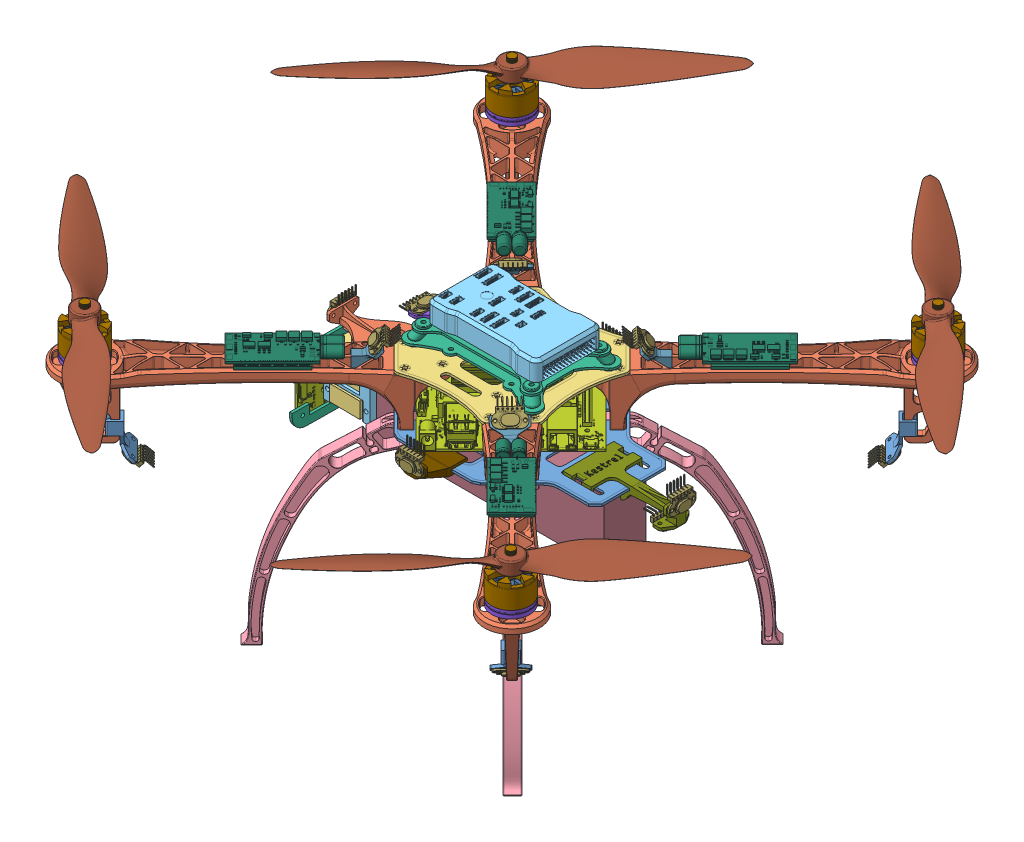
SolidWorks assembly KestrelAssem, configuration Default. Lengths in mm.
Overall size (525.79 228.99 525.79).
72 component instances, 26 part files, 118 mates.
Components (placement in the parent):
- Base bottom-1: Base bottom [Default] at (67.5563 86.9564 146.6689) size (182 1.6 118)
- arm-1: arm [Default] at (165.9237 126.3564 245.0469) x (-0.707107 0 0.707107) z (-0.707107 0 -0.707107) size (40.75 55.34 213.92)
- arm-2: arm [Default] at (-30.8217 126.3564 245.0362) x (-0.707107 0 -0.707107) z (0.707107 0 -0.707107) size (40.75 55.34 213.92)
- arm-3: arm [Default] at (165.9344 126.3564 48.3015) x (0.707107 0 0.707107) z (-0.707107 0 0.707107) size (40.75 55.34 213.92)
- arm-4: arm [Default] at (-30.811 126.3564 48.2908) x (0.707107 0 -0.707107) z (0.707107 0 0.707107) size (40.75 55.34 213.92)
- Base Top-1: Base Top [Default] at (67.5563 125.3865 146.6689) x (0 0 -1) z (1 0 0) size (108.15 1.65 108.15)
- patadrone3definitiva-1: patadrone3definitiva [Predeterminado] at (172.5269 -57.1369 48.4158) x (-0.707107 0 0.707107) z (-0.707107 0 -0.707107) size (111.61 160.57 31.98)
- patadrone3definitiva-2: patadrone3definitiva [Predeterminado] at (-30.3432 -57.1369 41.3447) x (0.707107 0 0.707107) z (-0.707107 0 0.707107) size (111.61 160.57 31.98)
- patadrone3definitiva-3: patadrone3definitiva [Predeterminado] at (165.8094 -57.1369 251.6394) x (-0.707107 0 -0.707107) z (0.707107 0 -0.707107) size (111.61 160.57 31.98)
- patadrone3definitiva-4: patadrone3definitiva [Predeterminado] at (-37.4142 -57.1369 244.9219) x (0.707107 0 -0.707107) z (0.707107 0 0.707107) size (111.61 160.57 31.98)
- pixhawk-1: pixhawk [Default] at (69.0326 138.9713 146.4116) x (0 0 1) z (-1 0 0) size (49.7 16 82)
- base_pixhawk-1: base_pixhawk [Predeterminado] at (67.5563 126.89 137.1312) x (0 0 -1) z (1 0 0) size (70 13.5 101)
- Jetson nano_fixed-2: Jetson nano_fixed [Default] at (50.0251 91.2381 194.8479) x (0.707107 0 -0.707107) z (0 1 0) size (100 81.03 30.51)
- emax2213-3: emax2213 [Default] at (-115.5179 114.2807 302.8982) x (0.53753 0 -0.843245) z (0.843245 0 0.53753) size (30.02 35.87 30.02)
  - Part27-1: Part27 [Default] at (10.7352 10.5257 21.811) size (27.95 6.6 27.95)
  - rotor-1: rotor [Default] at (10.7352 16.1257 21.811) x (-0.046958 0 -0.998897) z (0.998897 0 -0.046958) size (28.06 30.27 28.06)
  - stator-1: stator [Default] at (10.7352 14.6357 21.811) x (-0.821098 0 -0.570787) z (0.570787 0 -0.821098) size (21.57 13.8 21.57)
- Propeller 10x45-3: Propeller 10x45 [Default] at (-91.3554 152.6764 305.5699) x (0.684738 0 -0.72879) z (0.72879 0 0.684738) size (33.64 14.19 254.22)
- TOF400C-2: TOF400C [Défaut] at (16.6624 134.5984 197.0939) x (-0.726351 -0.001282 -0.687323) z (-0.486669 0.707107 0.512985) size (20 18.23 7.52)
- Battery-1: Battery [Default] at (67.5563 62.1564 131.356) x (1 0 0) z (0 -1 0) size (169 31.5 48)
- Top Sensor Mount-1: Top Sensor Mount [Default] at (14.5099 121.5155 199.3264) x (-0.688254 0 0.72547) z (-0.72547 0 -0.688254) size (17.07 22.27 22)
- ESC 26X50mm-1: ESC 26X50mm [Default] at (-21.2525 131.4243 235.9148) x (-0.707107 0 0.707107) z (0 1 0) size (62.87 25.9 10.08)
- Rear Horizontal Sensor Mount-1: Rear Horizontal Sensor Mount [Default] at (145.7563 87.8564 147.106) x (0 0 -1) z (1 0 0) size (39.5 19.31 69)
- TOF400C-8: TOF400C [Défaut] at (194.3563 93.7637 147.081) x (0 0 1) z (1 0 0) size (20 18.23 7.52)
- TOF400C-9: TOF400C [Défaut] at (67.5813 93.6637 68.2503) x (1 0 0) z (0 0 -1) size (20 18.23 7.52)
- Side Horizontal Mount-1: Side Horizontal Mount [Default] at (67.5563 87.7564 89.8503) x (-1 0 0) z (0 0 -1) size (26 12.61 27.76)
- Side Horizontal Mount Pt2-1: Side Horizontal Mount Pt2 [Default] at (67.5563 87.7564 199.3503) size (34.53 12.61 31.5)
- TOF400C-14: TOF400C [Défaut] at (67.5813 93.6637 222.9503) x (-1 0 0) z (0 0 1) size (20 18.23 7.52)
- Angle Down Mount-1: Angle Down Mount [Default] at (-82.2131 82.3894 291.9609) x (-0.707107 0 -0.707107) z (0.707107 0 -0.707107) size (22 23.82 16.77)
- TOF400C-15: TOF400C [Défaut] at (-74.539 64.8571 288.8477) x (0.707107 0 0.707107) z (-0.498006 -0.709916 0.498006) size (20 18.23 7.52)
- Forward Horizontal Sensor Mount-1: Forward Horizontal Sensor Mount [Default] at (-10.6437 87.8564 147.106) x (0 0 1) z (-1 0 0) size (40.84 19.31 71.66)
- TOF400C-19: TOF400C [Défaut] at (-59.2437 93.7637 147.081) x (0 0 -1) z (-1 0 0) size (20 18.23 7.52)
- SG90-servo-1: SG90-servo [Varsayılan] at (-47.0683 69.2064 147.0402) x (0.999938 0 0.011104) z (0 -1 0) size (33 11.95 30.5)
- Servo Arm-1: Servo Arm [Peça] at (-41.1437 84.1564 147.106) size (34.5 3.8 16.7)
- Camera Mount pt2-1: Camera Mount pt2 [Default] at (-61.5674 69.2064 146.8792) x (-0.999938 0 -0.011104) z (0.011104 0 -0.999938) size (35 33.25 15.8)
- SG90-servo-2: SG90-servo [Varsayılan] at (-46.9806 43.8564 139.1406) x (-0.999938 0 -0.011104) z (-0.011104 0 0.999938) size (33 11.95 30.5)
- Servo Arm-2: Servo Arm [Peça] at (-52.7392 43.8564 124.1258) x (-0.999816 -0.015644 -0.011102) z (0.015643 -0.999878 0.000174) size (34.5 3.8 16.7)
- Camera Mount Pt3-1: Camera Mount Pt3 [Default] at (-52.7392 43.8564 124.1258) x (0.011104 0 -0.999938) z (0.999816 0.015644 0.011102) size (49.7 49.7 38.4)
- Camera-1: Camera [Default] at (-74.4135 38.4187 136.2155) x (-0.015643 0.999878 -0.000174) z (-0.999816 -0.015644 -0.011102) size (38 38 23.66)
- Upward Sensor Mount-1: Upward Sensor Mount [Default] at (32.5563 126.2115 146.6689) x (0 0 1) z (-1 0 0) size (22 5.7 33.62)
- TOF400C-20: TOF400C [Défaut] at (3.699 126.9615 146.6439) x (0 0 1) z (0 1 0) size (20 18.23 7.52)
- TOF400C-21: TOF400C [Défaut] at (185.999 78.5564 147.081) x (0 0 -1) z (0 -1 0) size (20 18.23 7.52)
- TOF400C-5: TOF400C [Défaut] at (117.5443 134.5984 197.9999) x (-0.687323 -0.001282 0.726351) z (0.512985 0.707107 0.486669) size (20 18.23 7.52)
- TOF400C-6: TOF400C [Défaut] at (118.4503 134.5984 97.118) x (0.726351 -0.001282 0.687323) z (0.486669 0.707107 -0.512985) size (20 18.23 7.52)
- TOF400C-7: TOF400C [Défaut] at (17.5684 134.5984 96.212) x (0.687323 -0.001282 -0.726351) z (-0.512985 0.707107 -0.486669) size (20 18.23 7.52)
- Top Sensor Mount-2: Top Sensor Mount [Default] at (119.7768 121.5155 200.1524) x (0.72547 0 0.688254) z (-0.688254 0 0.72547) size (17.07 22.27 22)
- Top Sensor Mount-3: Top Sensor Mount [Default] at (120.6028 121.5155 94.8855) x (0.688254 0 -0.72547) z (0.72547 0 0.688254) size (17.07 22.27 22)
- Top Sensor Mount-4: Top Sensor Mount [Default] at (15.3359 121.5155 94.0595) x (-0.72547 0 -0.688254) z (0.688254 0 -0.72547) size (17.07 22.27 22)
- emax2213-5: emax2213 [Default] at (223.3486 114.2807 330.1802) x (-0.843245 0 -0.53753) z (0.53753 0 -0.843245) size (30.02 35.87 30.02)
  - Part27-1: Part27 [Default] at (10.7352 10.5257 21.811) size (27.95 6.6 27.95)
  - rotor-1: rotor [Default] at (10.7352 16.1257 21.811) x (-0.046958 0 -0.998897) z (0.998897 0 -0.046958) size (28.06 30.27 28.06)
  - stator-1: stator [Default] at (10.7352 14.6357 21.811) x (-0.821098 0 -0.570787) z (0.570787 0 -0.821098) size (21.57 13.8 21.57)
- emax2213-6: emax2213 [Default] at (250.6306 114.2807 -8.6863) x (-0.53753 0 0.843245) z (-0.843245 0 -0.53753) size (30.02 35.87 30.02)
  - Part27-1: Part27 [Default] at (10.7352 10.5257 21.811) size (27.95 6.6 27.95)
  - rotor-1: rotor [Default] at (10.7352 16.1257 21.811) x (-0.046958 0 -0.998897) z (0.998897 0 -0.046958) size (28.06 30.27 28.06)
  - stator-1: stator [Default] at (10.7352 14.6357 21.811) x (-0.821098 0 -0.570787) z (0.570787 0 -0.821098) size (21.57 13.8 21.57)
- emax2213-7: emax2213 [Default] at (-88.2359 114.2807 -35.9683) x (0.843245 0 0.53753) z (-0.53753 0 0.843245) size (30.02 35.87 30.02)
  - Part27-1: Part27 [Default] at (10.7352 10.5257 21.811) size (27.95 6.6 27.95)
  - rotor-1: rotor [Default] at (10.7352 16.1257 21.811) x (-0.046958 0 -0.998897) z (0.998897 0 -0.046958) size (28.06 30.27 28.06)
  - stator-1: stator [Default] at (10.7352 14.6357 21.811) x (-0.821098 0 -0.570787) z (0.570787 0 -0.821098) size (21.57 13.8 21.57)
- Propeller 10x45-5: Propeller 10x45 [Default] at (226.0203 152.6764 306.0177) x (-0.72879 0 -0.684738) z (0.684738 0 -0.72879) size (33.64 14.19 254.22)
- Propeller 10x45-6: Propeller 10x45 [Default] at (226.4681 152.6764 -11.358) x (-0.684738 0 0.72879) z (-0.72879 0 -0.684738) size (33.64 14.19 254.22)
- Propeller 10x45-7: Propeller 10x45 [Default] at (-90.9076 152.6764 -11.8058) x (0.72879 0 0.684738) z (-0.684738 0 0.72879) size (33.64 14.19 254.22)
- ESC 26X50mm-2: ESC 26X50mm [Default] at (156.3652 131.4243 235.9148) x (0.707107 0 0.707107) z (0 1 0) size (62.87 25.9 10.08)
- ESC 26X50mm-3: ESC 26X50mm [Default] at (156.3652 131.4243 58.2971) x (0.707107 0 -0.707107) z (0 1 0) size (62.87 25.9 10.08)
- ESC 26X50mm-4: ESC 26X50mm [Default] at (-21.2525 131.4243 58.2971) x (-0.707107 0 -0.707107) z (0 1 0) size (62.87 25.9 10.08)
- TOF400C-16: TOF400C [Défaut] at (-74.1854 64.8571 5.0106) x (-0.707107 0 0.707107) z (-0.498006 -0.709916 -0.498006) size (20 18.23 7.52)
- TOF400C-17: TOF400C [Défaut] at (209.6517 64.8571 5.3642) x (-0.707107 0 -0.707107) z (0.498006 -0.709916 -0.498006) size (20 18.23 7.52)
- TOF400C-18: TOF400C [Défaut] at (209.298 64.8571 289.2013) x (0.707107 0 -0.707107) z (0.498006 -0.709916 0.498006) size (20 18.23 7.52)
- Angle Down Mount-2: Angle Down Mount [Default] at (-77.2986 82.3894 -2.6635) x (0.707107 0 -0.707107) z (0.707107 0 0.707107) size (22 23.82 16.77)
- Angle Down Mount-3: Angle Down Mount [Default] at (217.3258 82.3894 2.251) x (0.707107 0 0.707107) z (-0.707107 0 0.707107) size (22 23.82 16.77)
- Angle Down Mount-4: Angle Down Mount [Default] at (212.4113 82.3894 296.8754) x (-0.707107 0 0.707107) z (-0.707107 0 -0.707107) size (22 23.82 16.77)
Mates (geometry in assembly coordinates):
- Coincident2: coincident anti-aligned: plane of Base bottom-1 through (4.0563 87.7564 186.9169) normal (0 1 0); plane of arm-1 through (104.3913 87.7564 193.9796) normal (0 -1 0)
- Coincident3: coincident anti-aligned: axis of Base bottom-1 through (99.5883 86.1554 193.1965) axis (0 1 0); line of arm-1 through (99.5883 92.7564 193.1965) axis (0 -1 0)
- Coincident4: coincident anti-aligned: line of Base bottom-1 through (114.084 86.1554 178.7008) axis (0 1 0); line of arm-1 through (114.084 92.7564 178.7008) axis (0 -1 0)
- Coincident5: coincident anti-aligned: plane of Base bottom-1 through (4.0563 87.7564 186.9169) normal (0 1 0); plane of arm-2 through (35.6249 87.7564 197.7501) normal (0 -1 0)
- Coincident6: coincident anti-aligned: line of Base bottom-1 through (21.0287 86.1554 178.7008) axis (0 1 0); line of arm-2 through (21.0287 92.7564 178.7008) axis (0 -1 0)
- Coincident7: coincident anti-aligned: line of Base bottom-1 through (35.5244 86.1554 193.1965) axis (0 1 0); line of arm-2 through (35.5244 92.7564 193.1965) axis (0 -1 0)
- Coincident8: coincident anti-aligned: line of Base bottom-1 through (114.084 86.1554 114.6369) axis (0 1 0); line of arm-3 through (114.084 92.7564 114.6369) axis (0 -1 0)
- Coincident9: coincident anti-aligned: plane of Base bottom-1 through (4.0563 87.7564 186.9169) normal (0 1 0); plane of arm-3 through (114.8671 87.7564 109.8339) normal (0 -1 0)
- Coincident10: coincident anti-aligned: line of Base bottom-1 through (99.5883 86.1554 100.1412) axis (0 1 0); line of arm-3 through (99.5883 92.7564 100.1412) axis (0 -1 0)
- Coincident13: coincident anti-aligned: line of Base bottom-1 through (35.5244 86.1554 100.1412) axis (0 1 0); line of arm-4 through (35.5244 92.7564 100.1412) axis (0 -1 0)
- Coincident14: coincident anti-aligned: plane of Base bottom-1 through (4.0563 87.7564 186.9169) normal (0 1 0); plane of arm-4 through (30.7214 87.7564 99.3581) normal (0 -1 0)
- Coincident15: coincident anti-aligned: line of Base bottom-1 through (21.0287 86.1554 114.6369) axis (0 1 0); line of arm-4 through (21.0287 92.7564 114.6369) axis (0 -1 0)
- Coincident16: coincident anti-aligned: plane of arm-1 through (121.2204 124.5615 177.999) normal (0 1 0); plane of Base Top-1 through (18.1568 124.5615 114.9285) normal (0 -1 0)
- Coincident17: coincident aligned: line of arm-1 through (99.0226 119.5615 194.7521) axis (0 1 0); line of Base Top-1 through (99.0226 124.5605 194.7521) axis (0 1 0)
- Coincident18: coincident aligned: line of arm-1 through (115.6396 119.5615 178.1351) axis (0 1 0); line of Base Top-1 through (115.6396 124.5605 178.1351) axis (0 1 0)
- Concentric1: concentric aligned: circle of Base bottom-1; circle of patadrone3definitiva-1
- Coincident19: coincident anti-aligned: plane of Base bottom-1 through (4.0563 86.1564 186.9169) normal (0 -1 0); plane of patadrone3definitiva-1 through (109.2957 86.1564 97.5049) normal (0 1 0)
- Parallel1: parallel aligned: line of Base bottom-1 through (123.9835 86.1564 115.344) axis (-0.707107 0 -0.707107); line of patadrone3definitiva-1 through (106.6908 86.1564 98.8433) axis (-0.707107 0 -0.707107)
- Concentric3: concentric aligned: circle of Base bottom-1; circle of patadrone3definitiva-2
- Coincident20: coincident anti-aligned: plane of Base bottom-1 through (4.0563 86.1564 186.9169) normal (0 -1 0); plane of patadrone3definitiva-2 through (18.7459 86.1564 104.576) normal (0 1 0)
- Parallel2: parallel aligned: line of Base bottom-1 through (30.9282 86.1564 95.545) axis (-0.707107 0 0.707107); line of patadrone3definitiva-2 through (32.7384 86.1564 94.5268) axis (-0.707107 0 0.707107)
- Concentric5: concentric aligned: circle of Base bottom-1; circle of patadrone3definitiva-4
- Coincident22: coincident anti-aligned: plane of Base bottom-1 through (4.0563 86.1564 186.9169) normal (0 -1 0); plane of patadrone3definitiva-4 through (25.817 86.1564 195.8328) normal (0 1 0)
- Parallel5: parallel aligned: line of Base bottom-1 through (12.0544 86.1564 178.9189) axis (0.707107 0 0.707107); line of patadrone3definitiva-4 through (28.4219 86.1564 194.4944) axis (0.707107 0 0.707107)
- Concentric6: concentric aligned: circle of Base bottom-1; circle of patadrone3definitiva-3
- Coincident23: coincident anti-aligned: plane of Base bottom-1 through (4.0563 86.1564 186.9169) normal (0 -1 0); plane of patadrone3definitiva-3 through (116.7203 86.1564 188.4082) normal (0 1 0)
- Parallel6: parallel aligned: line of Base bottom-1 through (99.8063 86.1564 202.1708) axis (0.707107 0 -0.707107); line of patadrone3definitiva-3 through (102.7278 86.1564 198.4574) axis (0.707107 0 -0.707107)
- Concentric7: concentric anti-aligned: circle of arm-3; circle of emax2213-1/Part27-1
- Coincident24: coincident anti-aligned: plane of arm-3 through (207.1853 124.8064 -19.441) normal (0 1 0); plane of emax2213-1/Part27-1 through (226.4681 124.8064 -12.2322) normal (0 -1 0)
- Concentric8: concentric anti-aligned: circle of arm-1; circle of emax2213-2/Part27-1
- Coincident25: coincident anti-aligned: plane of arm-1 through (233.6662 124.8064 286.2978) normal (0 1 0); plane of emax2213-2/Part27-1 through (226.4574 124.8064 305.5806) normal (0 -1 0)
- Concentric9: concentric anti-aligned: circle of arm-2; circle of emax2213-3/Part27-1
- Coincident26: coincident anti-aligned: plane of arm-2 through (-72.0726 124.8064 312.7787) normal (0 1 0); plane of emax2213-3/Part27-1 through (-91.3554 124.8064 305.5699) normal (0 -1 0)
- Concentric10: concentric anti-aligned: circle of arm-4; circle of emax2213-4/Part27-1
- Coincident27: coincident anti-aligned: plane of arm-4 through (-98.5535 124.8064 7.0399) normal (0 1 0); plane of emax2213-4/Part27-1 through (-91.3447 124.8064 -12.2429) normal (0 -1 0)
- Concentric11: concentric aligned: circle of emax2213-4/rotor-1; circle of Propeller 10x45-4
- Coincident28: coincident anti-aligned: plane of emax2213-4/rotor-1 through (-91.3447 147.6764 -12.2429) normal (0 1 0); plane of Propeller 10x45-4 through (-91.3447 147.6764 -12.2429) normal (0 -1 0)
- Concentric12: concentric aligned: circle of emax2213-3/rotor-1; circle of Propeller 10x45-3
- Coincident29: coincident anti-aligned: plane of emax2213-3/rotor-1 through (-91.3554 147.6764 305.5699) normal (0 1 0); plane of Propeller 10x45-3 through (-91.3554 147.6764 305.5699) normal (0 -1 0)
- Concentric13: concentric aligned: circle of emax2213-2/rotor-1; circle of Propeller 10x45-2
- Coincident30: coincident anti-aligned: plane of emax2213-2/rotor-1 through (226.4574 147.6764 305.5806) normal (0 1 0); plane of Propeller 10x45-2 through (226.4574 147.6764 305.5806) normal (0 -1 0)
- Concentric14: concentric aligned: circle of emax2213-1/rotor-1; circle of Propeller 10x45-1
- Coincident31: coincident anti-aligned: plane of emax2213-1/rotor-1 through (226.4681 147.6764 -12.2322) normal (0 1 0); plane of Propeller 10x45-1 through (226.4681 147.6764 -12.2322) normal (0 -1 0)
- Parallel8: parallel aligned: plane of Top Sensor Mount-1 through (14.5099 121.5155 199.3264) normal (0 1 0)
- Concentric15: concentric aligned: circle of TOF400C-2; circle of Top Sensor Mount-1
- Coincident37: coincident anti-aligned: plane of TOF400C-2 through (20.9493 134.1812 200.5664) normal (0.486669 -0.707107 -0.512985); plane of Top Sensor Mount-1 through (6.4052 136.3057 183.8399) normal (-0.486669 0.707107 0.512985)
- Coincident40: coincident: point of arm-2; line of ESC 26X50mm-1 through (-44.3113 125.4243 242.1277) axis (0.707107 0 0.707107)
- Coincident41: coincident: point of arm-2; line of ESC 26X50mm-1 through (-44.3113 125.4243 242.1277) axis (0.707107 0 0.707107)
- Parallel9: parallel anti-aligned: plane of ESC 26X50mm-1 through (-21.2243 125.4243 236.0113) normal (0 -1 0)
- Coincident42: coincident: line of ESC 26X50mm-1 through (-38.9301 131.4243 253.5924) axis (0.707107 0 -0.707107)
- Coincident43: coincident anti-aligned: plane of Base bottom-1 through (4.0563 86.1564 186.9169) normal (0 -1 0); plane of Battery-1 through (-16.9437 86.1564 162.856) normal (0 1 0)
- Coincident44: coincident anti-aligned: plane of Battery-1 through (67.5563 62.1564 131.356) normal (1 0 0)
- Distance1: distance = 15.75 mm aligned: plane of Battery-1 through (67.5563 62.1564 131.356) normal (0 0 1)
- Coincident46: coincident aligned: line of Base bottom-1 through (124.7563 86.1564 166.106) axis (1 0 0); line of Rear Horizontal Sensor Mount-1 through (138.7563 86.1564 166.106) axis (1 0 0)
- Coincident47: coincident anti-aligned: line of Base bottom-1 through (150.5563 86.1564 128.106) axis (-1 0 0); line of Rear Horizontal Sensor Mount-1 through (138.7563 86.1564 128.106) axis (1 0 0)
- Coincident48: coincident anti-aligned: plane of Battery-1 through (152.0563 86.1564 162.856) normal (1 0 0); plane of Rear Horizontal Sensor Mount-1 through (152.0563 84.1564 150.606) normal (-1 0 0)
- Concentric17: concentric aligned: circle of Rear Horizontal Sensor Mount-1; circle of TOF400C-8
- Coincident49: coincident anti-aligned: plane of Rear Horizontal Sensor Mount-1 through (193.7563 86.0064 110.1173) normal (1 0 0); plane of TOF400C-8 through (193.7563 93.7637 141.581) normal (-1 0 0)
- Parallel10: parallel anti-aligned: plane of Rear Horizontal Sensor Mount-1 through (191.7563 96.7637 147.106) normal (0 1 0); plane of TOF400C-8 through (191.2563 98.7237 154.501) normal (0 -1 0)
- Coincident50: coincident: point of Base bottom-1; point of Side Horizontal Mount-1
- Coincident51: coincident: point of Base bottom-1; point of Side Horizontal Mount-1
- Coincident52: coincident anti-aligned: plane of Base bottom-1 through (4.0563 87.7564 186.9169) normal (0 1 0); plane of Side Horizontal Mount-1 through (67.5563 87.7564 89.8503) normal (0 -1 0)
- Coincident53: coincident anti-aligned: plane of TOF400C-9 through (62.0813 93.6637 68.8503) normal (0 0 1); plane of Side Horizontal Mount-1 through (67.5563 87.7564 68.8503) normal (0 0 -1)
- Concentric18: concentric aligned: circle of TOF400C-9; circle of Side Horizontal Mount-1
- Parallel11: parallel anti-aligned: plane of TOF400C-9 through (62.3013 98.6237 71.3503) normal (0 -1 0); plane of Side Horizontal Mount-1 through (67.5563 96.6637 70.8503) normal (0 1 0)
- Coincident54: coincident: point of Base bottom-1; point of Side Horizontal Mount-3
- Coincident55: coincident: point of Base bottom-1; point of Side Horizontal Mount-3
- Coincident56: coincident anti-aligned: plane of Base bottom-1 through (4.0563 87.7564 186.9169) normal (0 1 0); plane of Side Horizontal Mount-3 through (67.5563 87.7564 199.3503) normal (0 -1 0)
- Coincident57: coincident: point of Base bottom-1; point of Side Horizontal Mount Pt2-1
- Coincident58: coincident: point of Base bottom-1; point of Side Horizontal Mount Pt2-1
- Coincident60: coincident anti-aligned: plane of Base bottom-1 through (4.0563 87.7564 186.9169) normal (0 1 0); plane of Side Horizontal Mount Pt2-1 through (67.5563 87.7564 199.3503) normal (0 -1 0)
- Concentric19: concentric aligned: circle of Side Horizontal Mount Pt2-1; circle of TOF400C-14
- Coincident61: coincident anti-aligned: plane of Side Horizontal Mount Pt2-1 through (67.5563 87.7564 222.3503) normal (0 0 1); plane of TOF400C-14 through (73.0813 93.6637 222.3503) normal (0 0 -1)
- Parallel12: parallel anti-aligned: plane of Side Horizontal Mount Pt2-1 through (67.5563 96.6637 220.3503) normal (0 1 0); plane of TOF400C-14 through (65.2413 98.6237 219.8503) normal (0 -1 0)
- Coincident64: coincident anti-aligned: line of arm-2 through (-79.7617 86.9894 298.0185) axis (-0.707107 0 -0.707107); line of Angle Down Mount-1 through (-84.0162 86.9894 293.7641) axis (0.707107 0 0.707107)
- Parallel14: parallel anti-aligned: plane of Angle Down Mount-1 through (-83.6273 77.7894 290.5467) normal (0 -1 0)
- Coincident68: coincident: plane of arm-2 through (-108.5911 119.3064 317.1488) normal (-0.706867 -0.026033 -0.706867); line of Angle Down Mount-1 through (-80.4453 86.9894 290.1932) axis (-0.707107 0 0.707107)
- Concentric20: concentric anti-aligned: circle of Angle Down Mount-1; circle of TOF400C-15
- Coincident69: coincident anti-aligned: plane of Angle Down Mount-1 through (-85.4373 77.7932 295.1852) normal (-0.498006 -0.709916 0.498006); plane of TOF400C-15 through (-78.1293 65.283 284.6598) normal (0.498006 0.709916 -0.498006)
- Parallel15: parallel anti-aligned: plane of Angle Down Mount-1 through (-74.0186 64.59 283.7665) normal (0.501986 -0.704287 -0.501986); plane of TOF400C-15 through (-74.2388 63.5646 281.0805) normal (-0.501986 0.704287 0.501986)
- Coincident70: coincident: point of Base bottom-1; point of Forward Horizontal Sensor Mount-1
- Coincident71: coincident: point of Base bottom-1; point of Forward Horizontal Sensor Mount-1
- Parallel16: parallel anti-aligned: plane of Base bottom-1 through (4.0563 87.7564 186.9169) normal (0 1 0); plane of Forward Horizontal Sensor Mount-1 through (-15.6437 87.8564 138.606) normal (0 -1 0)
- Concentric21: concentric aligned: circle of Forward Horizontal Sensor Mount-1; circle of TOF400C-19
- Coincident73: coincident anti-aligned: plane of Forward Horizontal Sensor Mount-1 through (-58.6437 86.0064 184.0946) normal (-1 0 0); plane of TOF400C-19 through (-58.6437 93.7637 152.581) normal (1 0 0)
- Parallel17: parallel anti-aligned: plane of Forward Horizontal Sensor Mount-1 through (-56.6437 96.7637 147.106) normal (0 1 0); plane of TOF400C-19 through (-56.1437 98.7237 144.741) normal (0 -1 0)
- Coincident74: coincident anti-aligned: plane of SG90-servo-1 through (-41.1437 82.3564 147.106) normal (0 1 0); plane of Servo Arm-1 through (-41.1437 82.3564 147.106) normal (0 -1 0)
- Concentric22: concentric anti-aligned: circle of SG90-servo-1; circle of Servo Arm-1
- Concentric23: concentric anti-aligned: circle of Forward Horizontal Sensor Mount-1; circle of Servo Arm-1
- Concentric24: concentric anti-aligned: circle of Forward Horizontal Sensor Mount-1; circle of Servo Arm-1
- Coincident75: coincident anti-aligned: plane of Forward Horizontal Sensor Mount-1 through (-10.6437 84.1564 147.106) normal (0 -1 0); plane of Servo Arm-1 through (-41.1437 84.1564 147.106) normal (0 1 0)
- Concentric25: concentric aligned: circle of SG90-servo-1; circle of Camera Mount pt2-1
- Coincident76: coincident anti-aligned: plane of SG90-servo-1 through (-58.5021 51.8564 141.0128) normal (-0.999938 0 -0.011104); plane of Camera Mount pt2-1 through (-58.5676 49.7564 146.9125) normal (0.999938 0 0.011104)
- Coincident77: coincident anti-aligned: plane of SG90-servo-1 through (-63.5018 69.2064 140.9573) normal (0 -1 0); plane of Camera Mount pt2-1 through (-61.5674 69.2064 146.8792) normal (0 1 0)
- Coincident78: coincident anti-aligned: plane of Camera Mount pt2-1 through (-61.4797 49.7564 138.9796) normal (0.011104 0 -0.999938); plane of SG90-servo-2 through (-30.4816 49.7564 139.3239) normal (-0.011104 0 0.999938)
- Concentric28: concentric anti-aligned: circle of Camera Mount pt2-1; circle of SG90-servo-2
- Concentric29: concentric aligned: circle of Camera Mount pt2-1; circle of SG90-servo-2
- Coincident79: coincident anti-aligned: plane of SG90-servo-2 through (-52.7592 43.8564 125.9257) normal (0.011104 0 -0.999938); plane of Servo Arm-2 through (-52.7592 43.8564 125.9257) normal (-0.011104 0 0.999938)
- Concentric30: concentric anti-aligned: circle of SG90-servo-2; circle of Servo Arm-2
- Concentric31: concentric aligned: circle of Servo Arm-2; circle of Camera Mount Pt3-1
- Concentric32: concentric aligned: circle of Servo Arm-2; circle of Camera Mount Pt3-1
- Coincident80: coincident anti-aligned: plane of Servo Arm-2 through (-52.7392 43.8564 124.1258) normal (0.011104 0 -0.999938); plane of Camera Mount Pt3-1 through (-52.7392 43.8564 124.1258) normal (-0.011104 0 0.999938)
- Coincident81: coincident anti-aligned: plane of Camera Mount Pt3-1 through (-72.6633 43.5443 121.9044) normal (-0.999816 -0.015644 -0.011102); plane of Arducam B0332.stp-1 through (-73.5904 43.9425 147.7969) normal (0.969091 0.245945 -0.019351)
- Parallel18: parallel aligned: plane of Camera Mount Pt3-1 through (-52.7232 48.7976 122.4822) normal (0.152848 0.988245 -0.003052); plane of Arducam B0332.stp-1 through (-77.8944 62.4074 166.9366) normal (-0.245896 0.969284 0.00491)
- Coincident87: coincident anti-aligned: plane of Camera Mount Pt3-1 through (-72.6633 43.5443 121.9044) normal (-0.999816 -0.015644 -0.011102); plane of Camera-1 through (-72.8308 24.5466 163.7551) normal (0.999816 0.015644 0.011102)
- Coincident88: coincident anti-aligned: line of Camera Mount Pt3-1 through (-73.3697 62.5419 158.7488) axis (0.011104 0 -0.999938); line of Camera-1 through (-73.0477 62.5419 129.7506) axis (-0.011104 0 0.999938)
- Coincident89: coincident anti-aligned: line of Camera Mount Pt3-1 through (-72.916 55.5428 127.752) axis (0.015643 -0.999878 0.000174); line of Camera-1 through (-72.4624 26.5463 127.757) axis (-0.015643 0.999878 -0.000174)
- Coincident90: coincident: line of base_pixhawk-1 through (67.5563 130.1863 165.2343) axis (0 0 -1)
- Coincident91: coincident: line of base_pixhawk-1 through (31.3063 130.1863 147.106) axis (1 0 0)
- Coincident92: coincident aligned: line of Base Top-1 through (32.5563 126.2115 138.1689) axis (0 0 1); line of Upward Sensor Mount-1 through (32.5563 126.2115 138.1689) axis (0 0 1)
- Coincident93: coincident: point of Base Top-1; point of Upward Sensor Mount-1
- Coincident94: coincident anti-aligned: plane of Base Top-1 through (18.1568 126.2115 114.9285) normal (0 1 0); plane of Upward Sensor Mount-1 through (32.5563 126.2115 146.6689) normal (0 -1 0)
- Concentric33: concentric anti-aligned: circle of Upward Sensor Mount-1; circle of TOF400C-20
- Coincident95: coincident anti-aligned: plane of Upward Sensor Mount-1 through (32.5563 126.3615 146.6689) normal (0 1 0); plane of TOF400C-20 through (3.699 126.3615 141.1439) normal (0 -1 0)
- Parallel19: parallel anti-aligned: plane of Upward Sensor Mount-1 through (0.699 124.3615 146.6689) normal (-1 0 0); plane of TOF400C-20 through (-1.261 123.8615 154.0639) normal (1 0 0)
- Concentric37: concentric aligned: circle of Rear Horizontal Sensor Mount-1; circle of TOF400C-21
- Coincident99: coincident anti-aligned: plane of Rear Horizontal Sensor Mount-1 through (145.7563 79.1564 147.106) normal (0 -1 0); plane of TOF400C-21 through (185.999 79.1564 152.581) normal (0 1 0)
- Parallel22: parallel anti-aligned: plane of Rear Horizontal Sensor Mount-1 through (182.999 79.1564 147.106) normal (-1 0 0); plane of TOF400C-21 through (181.039 81.6564 152.361) normal (1 0 0)
